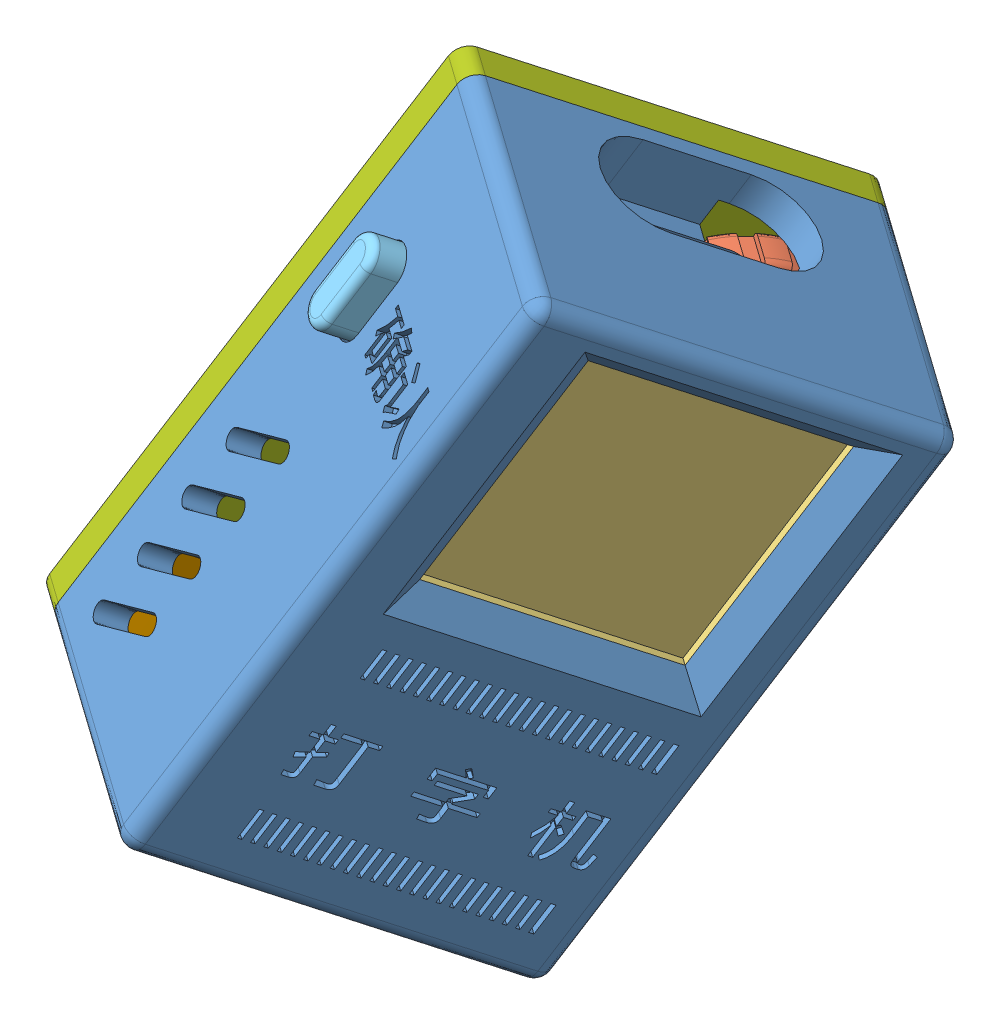
SolidWorks assembly 装配结果, configuration 默认. Lengths in mm.
Overall size (39.96 47.43 42.89).
10 component instances, 10 part files, 30 mates.
Components (placement in the parent):
- 底壳-1: 底壳 [默认] at (-149.4728 -161.4638 86.1808) x (-0.386865 -0.850817 0.355593) z (0.40861 -0.50386 -0.761028) size (38 16.45 24.5)
- 滚轮-1: 滚轮 [默认] at (-116.6898 -135.6126 13.9225) x (0.40861 -0.50386 -0.761028) z (-0.386865 -0.850817 0.355593) size (14.01 4.03 14.04)
- 屏幕-1: 屏幕 [默认] at (-120.0288 -116.1839 48.1247) x (0.40861 -0.50386 -0.761028) z (-0.386865 -0.850817 0.355593) size (17.6 9.86 34.5)
- 金属方轴-1: 金属方轴 [默认] at (-124.5693 -119.7216 37.2506) x (0.40861 -0.50386 -0.761028) z (-0.386865 -0.850817 0.355593) size (0.8 5.4 0.8)
- 按钮-1: 按钮 [默认] at (-132.1068 -108.162 50.6878) x (-0.386865 -0.850817 0.355593) z (-0.40861 0.50386 0.761028) size (11.5 4 4)
- 电池2-1: 电池2 [默认] at (-129.2572 -134.0457 57.276) x (0.40861 -0.50386 -0.761028) z (-0.826664 0.149116 -0.542578) size (20 33.5 4.2)
- 盖子2-1: 盖子2 [默认] at (-202.6306 -117.6275 148.9006) x (-0.40861 0.50386 0.761028) z (-0.826664 0.149116 -0.542578) size (24.5 38 7)
- 天线-1: 天线 [默认] at (-139.7053 -132.9385 63.3763) x (-0.40861 0.50386 0.761028) z (0.386865 0.850817 -0.355593) size (20.5 8.16 12.5)
- 震动模块-1: 震动模块 [默认] at (-130.2584 -137.6406 62.4036) x (0.802117 -0.500721 -0.325402) z (0.386865 0.850817 -0.355593) size (8 8 4)
- 3D_生产板_2025-07-1222-1: 3D_生产板_2025-07-1222 [默认] at (-116.5004 -108.9138 32.3983) x (-0.40861 0.50386 0.761028) z (-0.826664 0.149116 -0.542578) size (19.67 25.38 6.55)
Mates (geometry in assembly coordinates):
- 重合24: coincident: line of 底壳-1 through (-118.9893 -128.9892 45.8968) axis (0.386865 0.850817 -0.355593); plane of 屏幕-1 through (-113.5184 -115.9738 40.217) normal (-0.40861 0.50386 0.761028)
- 重合26: coincident: line of 底壳-1 through (-113.1051 -116.0483 40.4883) axis (-0.40861 0.50386 0.761028); plane of 屏幕-1 through (-119.7333 -108.31 51.7922) normal (-0.386865 -0.850817 0.355593)
- 重合37: coincident anti-aligned: plane of 底壳-1 through (-150.7128 -161.2401 85.3669) normal (-0.826664 0.149116 -0.542578); plane of 屏幕-1 through (-118.7392 -116.4165 48.9712) normal (0.826664 -0.149116 0.542578)
- 重合58: coincident: plane of 底壳-1 through (-122.5913 -113.1119 28.1947) normal (0.40861 -0.50386 -0.761028); line of 盖子-1 through (-123.365 -114.8135 28.9059) axis (-0.386865 -0.850817 0.355593)
- 重合61: coincident anti-aligned: plane of 滚轮-1 through (-116.6898 -135.6126 13.9225) normal (0.826664 -0.149116 0.542578); plane of 金属方轴-1 through (-127.9987 -119.8395 35.4874) normal (-0.826664 0.149116 -0.542578)
- 重合62: coincident anti-aligned: plane of 滚轮-1 through (-127.6814 -119.1418 35.1958) normal (0.40861 -0.50386 -0.761028); plane of 金属方轴-1 through (-123.5347 -120.6447 38.4173) normal (-0.40861 0.50386 0.761028)
- 重合63: coincident anti-aligned: plane of 滚轮-1 through (-127.9987 -119.8395 35.4874) normal (0.386865 0.850817 -0.355593); plane of 金属方轴-1 through (-124.8788 -120.4022 37.5351) normal (-0.386865 -0.850817 0.355593)
- 重合78: coincident anti-aligned: plane of 底壳-1 through (-125.6713 -134.2205 41.8306) normal (-0.40861 0.50386 0.761028); plane of 电池-1 through (-128.3264 -142.027 45.5735) normal (0.40861 -0.50386 -0.761028)
- 重合79: coincident anti-aligned: plane of 底壳-1 through (-155.6314 -160.3529 82.1386) normal (-0.826664 0.149116 -0.542578); plane of 电池-1 through (-130.5527 -133.8401 51.2155) normal (0.826664 -0.149116 0.542578)
- 重合80: coincident anti-aligned: plane of 底壳-1 through (-126.0799 -133.7167 42.5916) normal (-0.386865 -0.850817 0.355593); plane of 电池-1 through (-124.0709 -132.668 41.662) normal (0.386865 0.850817 -0.355593)
- 重合82: coincident anti-aligned: plane of 底壳-1 through (-133.7622 -114.2616 53.8374) normal (0.40861 -0.50386 -0.761028); plane of 按钮-1 through (-132.1068 -108.162 50.6878) normal (-0.40861 0.50386 0.761028)
- 平行4: parallel anti-aligned: plane of 底壳-1 through (-132.3254 -112.1569 54.5306) normal (-0.826664 0.149116 -0.542578); plane of 按钮-1 through (-131.7909 -108.0793 54.7447) normal (0.826664 -0.149116 0.542578)
- 距离2: distance = 0 mm: cylinder of 按钮-1 through (-132.7829 -107.9003 54.0936) axis (0.40861 -0.50386 -0.761028) radius 1.2; cylinder of 底壳-1 through (-131.9661 -108.9076 52.5723) axis (0.40861 -0.50386 -0.761028) radius 1.25
- 重合105: coincident anti-aligned: plane of 底壳-1 through (-113.0636 -115.8114 37.7256) normal (-0.40861 0.50386 0.761028); plane of 电池2-1 through (-129.5452 -143.6785 47.3266) normal (0.40861 -0.50386 -0.761028)
- 重合100: coincident anti-aligned: plane of 底壳-1 through (-163.0714 -159.0108 77.2554) normal (-0.826664 0.149116 -0.542578); plane of 盖子2-1 through (-202.6306 -117.6275 148.9006) normal (0.826664 -0.149116 0.542578)
- 重合101: coincident aligned: plane of 底壳-1 through (-122.5913 -113.1119 28.1947) normal (0.40861 -0.50386 -0.761028); plane of 盖子2-1 through (-124.2446 -112.8136 27.1096) normal (0.40861 -0.50386 -0.761028)
- 重合102: coincident aligned: plane of 底壳-1 through (-137.2921 -145.4429 41.7072) normal (-0.386865 -0.850817 0.355593); plane of 盖子2-1 through (-148.9564 -132.8001 59.2673) normal (-0.386865 -0.850817 0.355593)
- 重合106: coincident anti-aligned: plane of 底壳-1 through (-121.4401 -105.4822 53.3267) normal (-0.386865 -0.850817 0.355593); plane of 电池2-1 through (-124.7574 -105.0989 50.6348) normal (0.386865 0.850817 -0.355593)
- 重合108: coincident anti-aligned: plane of 屏幕-1 through (-120.0288 -116.1839 48.1247) normal (-0.826664 0.149116 -0.542578); plane of 电池2-1 through (-129.2572 -134.0457 57.276) normal (0.826664 -0.149116 0.542578)
- 重合118: coincident anti-aligned: plane of 底壳-1 through (-134.5935 -134.41 65.4169) normal (0.386865 0.850817 -0.355593); plane of 震动模块-1 through (-141.2882 -134.9284 56.8931) normal (-0.386865 -0.850817 0.355593)
- 重合119: coincident anti-aligned: plane of 底壳-1 through (-126.1437 -120.5042 42.3574) normal (-0.826664 0.149116 -0.542578); plane of 3D_生产板_2025-07-1222-1 through (-125.1472 -114.1188 42.5941) normal (0.826664 -0.149116 0.542578)
- 平行9: parallel anti-aligned: plane of 底壳-1 through (-121.4401 -105.4822 53.3267) normal (0.40861 -0.50386 -0.761028); plane of 3D_生产板_2025-07-1222-1 through (-127.4563 -107.5319 49.4702) normal (-0.40861 0.50386 0.761028)
- 重合122: coincident anti-aligned: plane of 底壳-1 through (-123.9494 -108.9756 49.8312) normal (-0.386865 -0.850817 0.355593); plane of 3D_生产板_2025-07-1222-1 through (-119.6965 -117.1005 35.0178) normal (0.386865 0.850817 -0.355593)
- 重合123: coincident anti-aligned: plane of 金属方轴-1 through (-123.2078 -121.0478 37.8085) normal (0.40861 -0.50386 -0.761028); plane of 3D_生产板_2025-07-1222-1 through (-125.2921 -120.5932 36.3884) normal (-0.40861 0.50386 0.761028)
- 重合124: coincident anti-aligned: plane of 金属方轴-1 through (-123.5347 -120.6447 38.4173) normal (0.826664 -0.149116 0.542578); plane of 3D_生产板_2025-07-1222-1 through (-128.8796 -122.4059 46.0768) normal (-0.826664 0.149116 -0.542578)
- 重合125: coincident anti-aligned: plane of 金属方轴-1 through (-124.8788 -120.4022 37.5351) normal (-0.386865 -0.850817 0.355593); plane of 3D_生产板_2025-07-1222-1 through (-125.5693 -120.3647 36.8736) normal (0.386865 0.850817 -0.355593)
- 重合126: coincident anti-aligned: plane of 底壳-1 through (-113.0636 -115.8114 37.7256) normal (-0.40861 0.50386 0.761028); plane of 3D_生产板_2025-07-1222-1 through (-128.9805 -137.5185 43.5514) normal (0.40861 -0.50386 -0.761028)
- 重合127: coincident anti-aligned: plane of 底壳-1 through (-151.9528 -161.0164 84.553) normal (-0.826664 0.149116 -0.542578); plane of 天线-1 through (-126.128 -144.5435 49.734) normal (0.826664 -0.149116 0.542578)
- 重合128: coincident anti-aligned: plane of 底壳-1 through (-113.0636 -115.8114 37.7256) normal (-0.40861 0.50386 0.761028); plane of 天线-1 through (-126.128 -144.5435 49.734) normal (0.40861 -0.50386 -0.761028)
- 重合129: coincident anti-aligned: plane of 底壳-1 through (-134.5935 -134.41 65.4169) normal (0.386865 0.850817 -0.355593); plane of 天线-1 through (-139.7053 -132.9385 63.3763) normal (-0.386865 -0.850817 0.355593)
